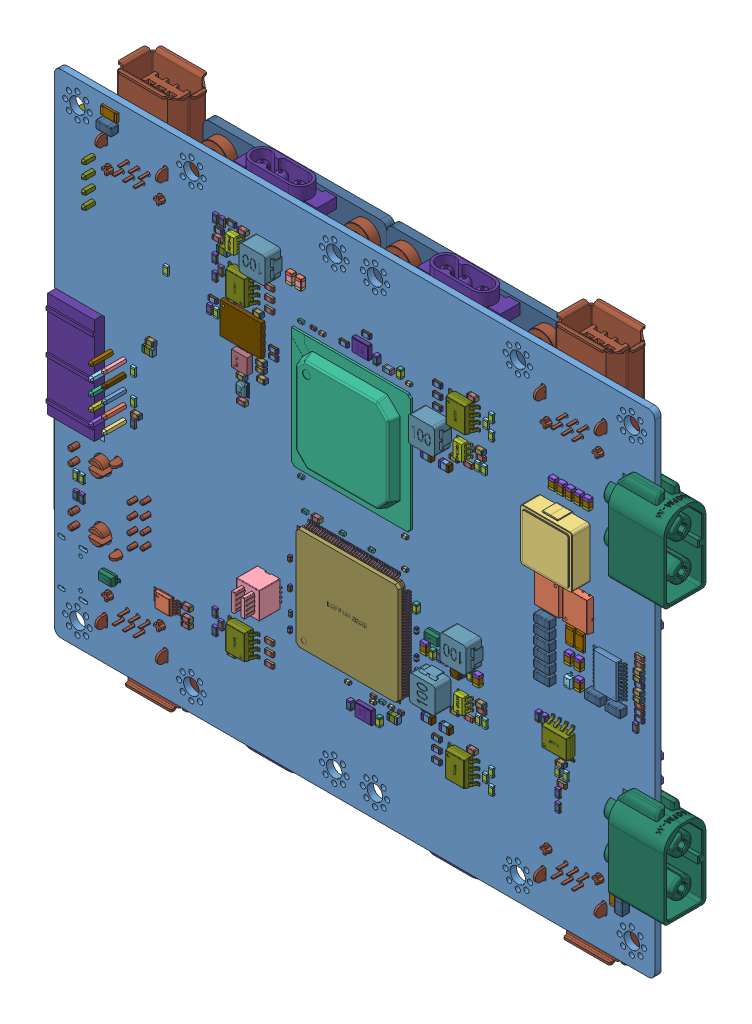
SolidWorks assembly Mother  Board, configuration 默认. Lengths in mm. (continued)
Components (placement in the parent): (continued)
- Mother  Board.step-1: Mother  Board.step [默认] at origin size (122.6 102.08 21) (continued)
  - C26.step-1: C26.step [默认] at origin size (1.6 0.8 0.8) (continued)
    - 5993854224.step-1: 5993854224.step [默认] at (32.3851 81.5341 0) x (1 0 0) z (0 0 1) size (1.6 0.8 0.8) (continued)
      - Terminal-17.step-1: Terminal-17.step [默认] at (-0.8 -0.4 0) size (1.6 0.8 0.8)
        - Open_CASCADE_STEP_translator_6.8_47.1.1-60.step-1: Open_CASCADE_STEP_translator_6.8_47.1.1-60.step [默认] at origin size (0.3 0.8 0.8)
        - Open_CASCADE_STEP_translator_6.8_47.1.2-61.step-1: Open_CASCADE_STEP_translator_6.8_47.1.2-61.step [默认] at origin size (0.3 0.8 0.8)
      - Mid_Body-8.step-1: Mid_Body-8.step [默认] at (-0.8 -0.4 0) size (1 0.8 0.8)
        - Open_CASCADE_STEP_translator_6.8_47.2.1-62.step-1: Open_CASCADE_STEP_translator_6.8_47.2.1-62.step [默认] at origin size (1 0.8 0.8)
  - C25.step-1: C25.step [默认] at origin size (2.01 1.25 0.94)
    - 5993850544.step-1: 5993850544.step [默认] at (28.7019 76.5809 0) x (-1 0 0) z (0 0 1) size (2.01 1.25 0.94)
      - Fillet1-63.step-1: Fillet1-63.step [默认] at origin size (0.5 1.25 0.94)
      - Fillet2-64.step-1: Fillet2-64.step [默认] at origin size (0.5 1.25 0.94)
      - body2-65.step-1: body2-65.step [默认] at origin size (1.01 1.22 0.92)
  - C24.step-1: C24.step [默认] at origin size (1.6 0.8 0.8)
    - 5993853264.step-1: 5993853264.step [默认] at (73.4059 21.8439 0) x (-1 0 0) z (0 0 1) size (1.6 0.8 0.8)
      - Terminal-6.step-1: Terminal-6.step [默认] at (-0.8 -0.4 0) size (1.6 0.8 0.8)
        - Open_CASCADE_STEP_translator_6.8_47.1.1-10.step-1: Open_CASCADE_STEP_translator_6.8_47.1.1-10.step [默认] at origin size (0.3 0.8 0.8)
        - Open_CASCADE_STEP_translator_6.8_47.1.2-11.step-1: Open_CASCADE_STEP_translator_6.8_47.1.2-11.step [默认] at origin size (0.3 0.8 0.8)
      - Mid_Body-5.step-1: Mid_Body-5.step [默认] at (-0.8 -0.4 0) size (1 0.8 0.8)
        - Open_CASCADE_STEP_translator_6.8_47.2.1-12.step-1: Open_CASCADE_STEP_translator_6.8_47.2.1-12.step [默认] at origin size (1 0.8 0.8)
  - C23.step-1: C23.step [默认] at origin size (2.01 1.25 0.94)
    - 5993850784.step-1: 5993850784.step [默认] at (71.6281 18.1611 0) x (1 0 0) z (0 0 1) size (2.01 1.25 0.94)
      - Fillet1.step-1: Fillet1.step [默认] at origin size (0.5 1.25 0.94)
      - Fillet2.step-1: Fillet2.step [默认] at origin size (0.5 1.25 0.94)
      - body2.step-1: body2.step [默认] at origin size (1.01 1.22 0.92)
  - C21.step-1: C21.step [默认] at origin size (2.01 1.25 0.94)
    - 5993850784.step-1: 5993850784.step [默认] at (68.0721 63.6271 0) x (1 0 0) z (0 0 1) size (2.01 1.25 0.94)
      - Fillet1.step-1: Fillet1.step [默认] at origin size (0.5 1.25 0.94)
      - Fillet2.step-1: Fillet2.step [默认] at origin size (0.5 1.25 0.94)
      - body2.step-1: body2.step [默认] at origin size (1.01 1.22 0.92)
  - C19.step-1: C19.step [默认] at origin size (1.25 2.01 0.94)
    - 5993850384.step-1: 5993850384.step [默认] at (43.4341 78.4859 0) x (0 -1 0) z (0 0 1) size (2.01 1.25 0.94)
      - Fillet1-51.step-1: Fillet1-51.step [默认] at origin size (0.5 1.25 0.94)
      - Fillet2-52.step-1: Fillet2-52.step [默认] at origin size (0.5 1.25 0.94)
      - body2-53.step-1: body2-53.step [默认] at origin size (1.01 1.22 0.92)
  - C17.step-1: C17.step [默认] at origin size (2.01 1.25 0.94)
    - 5993850784.step-1: 5993850784.step [默认] at (68.1991 18.1611 0) x (1 0 0) z (0 0 1) size (2.01 1.25 0.94)
      - Fillet1.step-1: Fillet1.step [默认] at origin size (0.5 1.25 0.94)
      - Fillet2.step-1: Fillet2.step [默认] at origin size (0.5 1.25 0.94)
      - body2.step-1: body2.step [默认] at origin size (1.01 1.22 0.92)
  - C16.step-1: C16.step [默认] at origin size (1.6 0.8 0.8)
    - 5993853264.step-1: 5993853264.step [默认] at (78.1049 67.6909 0) x (-1 0 0) z (0 0 1) size (1.6 0.8 0.8)
      - Terminal-6.step-1: Terminal-6.step [默认] at (-0.8 -0.4 0) size (1.6 0.8 0.8)
        - Open_CASCADE_STEP_translator_6.8_47.1.1-10.step-1: Open_CASCADE_STEP_translator_6.8_47.1.1-10.step [默认] at origin size (0.3 0.8 0.8)
        - Open_CASCADE_STEP_translator_6.8_47.1.2-11.step-1: Open_CASCADE_STEP_translator_6.8_47.1.2-11.step [默认] at origin size (0.3 0.8 0.8)
      - Mid_Body-5.step-1: Mid_Body-5.step [默认] at (-0.8 -0.4 0) size (1 0.8 0.8)
        - Open_CASCADE_STEP_translator_6.8_47.2.1-12.step-1: Open_CASCADE_STEP_translator_6.8_47.2.1-12.step [默认] at origin size (1 0.8 0.8)
  - C15.step-1: C15.step [默认] at origin size (1.6 0.8 0.8)
    - 5993854224.step-1: 5993854224.step [默认] at (27.5591 77.9781 0) x (1 0 0) z (0 0 1) size (1.6 0.8 0.8)
      - Terminal-17.step-1: Terminal-17.step [默认] at (-0.8 -0.4 0) size (1.6 0.8 0.8)
        - Open_CASCADE_STEP_translator_6.8_47.1.1-60.step-1: Open_CASCADE_STEP_translator_6.8_47.1.1-60.step [默认] at origin size (0.3 0.8 0.8)
        - Open_CASCADE_STEP_translator_6.8_47.1.2-61.step-1: Open_CASCADE_STEP_translator_6.8_47.1.2-61.step [默认] at origin size (0.3 0.8 0.8)
      - Mid_Body-8.step-1: Mid_Body-8.step [默认] at (-0.8 -0.4 0) size (1 0.8 0.8)
        - Open_CASCADE_STEP_translator_6.8_47.2.1-62.step-1: Open_CASCADE_STEP_translator_6.8_47.2.1-62.step [默认] at origin size (1 0.8 0.8)
  - C14.step-1: C14.step [默认] at origin size (1.6 0.8 0.8)
    - 5993853264.step-1: 5993853264.step [默认] at (78.2319 25.3999 0) x (-1 0 0) z (0 0 1) size (1.6 0.8 0.8)
      - Terminal-6.step-1: Terminal-6.step [默认] at (-0.8 -0.4 0) size (1.6 0.8 0.8)
        - Open_CASCADE_STEP_translator_6.8_47.1.1-10.step-1: Open_CASCADE_STEP_translator_6.8_47.1.1-10.step [默认] at origin size (0.3 0.8 0.8)
        - Open_CASCADE_STEP_translator_6.8_47.1.2-11.step-1: Open_CASCADE_STEP_translator_6.8_47.1.2-11.step [默认] at origin size (0.3 0.8 0.8)
      - Mid_Body-5.step-1: Mid_Body-5.step [默认] at (-0.8 -0.4 0) size (1 0.8 0.8)
        - Open_CASCADE_STEP_translator_6.8_47.2.1-12.step-1: Open_CASCADE_STEP_translator_6.8_47.2.1-12.step [默认] at origin size (1 0.8 0.8)
  - X1.step-1: X1.step [默认] at origin size (3.2 2.5 0.8)
    - XTAL-3225.step-1: XTAL-3225.step [默认] at (23.9389 30.1217 -1.2164) x (0 -1 0) z (1 0 0) size (2.5 0.8 3.2)
  - U12.step-1: U12.step [默认] at origin size (5.03 3.01 1.05)
    - User_Library-MSOP-10-1.step-1: User_Library-MSOP-10-1.step [默认] at (17.3989 12.0603 0) x (0 -1 0) z (-1 0 0) size (3.01 1.05 5.03)
  - U11.step-1: U11.step [默认] at origin size (4.02 4.02 1.08)
    - User_Library-QFN24_4x4.step-1: User_Library-QFN24_4x4.step [默认] at (21.844 21.3359 -1.2164) x (0 -1 0) z (0 0 -1) size (4.02 4.02 1.08)
      - Imported.step-1: Imported.step [默认] at origin size (2.5 2.5 0.02)
      - Imported_2.step-1: Imported_2.step [默认] at origin size (0.42 0.25 0.1)
      - Imported_3.step-1: Imported_3.step [默认] at origin size (0.42 0.25 0.1)
      - Imported_4.step-1: Imported_4.step [默认] at origin size (0.42 0.25 0.1)
      - Imported_5.step-1: Imported_5.step [默认] at origin size (0.42 0.25 0.1)
      - Imported_6.step-1: Imported_6.step [默认] at origin size (0.42 0.25 0.1)
      - Imported_7.step-1: Imported_7.step [默认] at origin size (0.42 0.25 0.1)
      - Imported_8.step-1: Imported_8.step [默认] at origin size (0.42 0.25 0.1)
      - Imported_9.step-1: Imported_9.step [默认] at origin size (0.42 0.25 0.1)
      - Imported_10.step-1: Imported_10.step [默认] at origin size (0.42 0.25 0.1)
      - Imported_11.step-1: Imported_11.step [默认] at origin size (0.42 0.25 0.1)
      - Imported_12.step-1: Imported_12.step [默认] at origin size (0.42 0.25 0.1)
      - Imported_13.step-1: Imported_13.step [默认] at origin size (0.42 0.25 0.1)
      - Imported_14.step-1: Imported_14.step [默认] at origin size (0.25 0.42 0.1)
      - Imported_15.step-1: Imported_15.step [默认] at origin size (0.25 0.42 0.1)
      - Imported_16.step-1: Imported_16.step [默认] at origin size (0.25 0.42 0.1)
      - Imported_17.step-1: Imported_17.step [默认] at origin size (0.25 0.42 0.1)
      - Imported_18.step-1: Imported_18.step [默认] at origin size (0.25 0.42 0.1)
      - Imported_19.step-1: Imported_19.step [默认] at origin size (0.25 0.42 0.1)
      - Imported_20.step-1: Imported_20.step [默认] at origin size (0.25 0.42 0.1)
      - Imported_21.step-1: Imported_21.step [默认] at origin size (0.25 0.42 0.1)
      - Imported_22.step-1: Imported_22.step [默认] at origin size (0.25 0.42 0.1)
      - Imported_23.step-1: Imported_23.step [默认] at origin size (0.25 0.42 0.1)
      - Imported_24.step-1: Imported_24.step [默认] at origin size (0.25 0.42 0.1)
      - Imported_25.step-1: Imported_25.step [默认] at origin size (0.25 0.42 0.1)
      - Imported_26.step-1: Imported_26.step [默认] at origin size (4 4 0.08)
      - Imported_27.step-1: Imported_27.step [默认] at origin size (3.85 3.85 0.9)
      - Imported_28.step-1: Imported_28.step [默认] at origin size (0.48 0.46 1.02)
  - U9.step-1: U9.step [默认] at origin size (3.02 3.02 1.05)
    - User_Library-MPU9250.step-1: User_Library-MPU9250.step [默认] at (32.2581 59.8168 0.03) x (0 -1 0) z (-1 0 0) size (3.02 1.05 3.02)
  - U8.step-1: U8.step [默认] at origin size (2 2.5 1)
    - User_Library-BST-BMP280.step-1: User_Library-BST-BMP280.step [默认] at (32.2581 55.1181 0) x (0 1 0) z (1 0 0) size (2.5 1 2)
  - U7.step-1: U7.step [默认] at origin size (5 6.01 1.9)
    - SOP8.step-1: SOP8.step [默认] at (93.809 27.432 0) x (0 1 0) z (0 0 1) size (6.01 5 1.9)
      - LOGO_-69.step-1: LOGO_-69.step [默认] at (0.0116 0 0.095) x (0 -1 0) z (0 0 -1) size (1.5 1.73 0.01)
      - SOP8-70.step-1: SOP8-70.step [默认] at origin size (6.01 5 1.9)
  - U6.step-1: U6.step [默认] at origin size (2.8 2.9 1.1)
    - User_Library-SOT23-5.step-1: User_Library-SOT23-5.step [默认] at (74.6706 27.9029 -0.15) x (0 1 0) z (1 0 0) size (2.9 1.1 2.8)
      - User_Library-SOT23-5_SOT23-5_Connector_Default.step-1: User_Library-SOT23-5_SOT23-5_Connector_Default.step [默认] at (0.2717 0.137 -1.6839) x (0 0 -1) z (1 0 0) size (0.6 0.85 0.43)
      - User_Library-SOT23-5_SOT23-5_Connector_Default.step-2: User_Library-SOT23-5_SOT23-5_Connector_Default.step [默认] at (2.1716 0.137 -1.6839) x (0 0 -1) z (1 0 0) size (0.6 0.85 0.43)
      - User_Library-SOT23-5_SOT23-5_Connector_Default.step-3: User_Library-SOT23-5_SOT23-5_Connector_Default.step [默认] at (2.597 0.137 -0.0849) x (0 0 1) z (-1 0 0) size (0.6 0.85 0.43)
      - User_Library-SOT23-5_SOT23-5_Connector_Default.step-4: User_Library-SOT23-5_SOT23-5_Connector_Default.step [默认] at (0.6971 0.137 -0.0849) x (0 0 1) z (-1 0 0) size (0.6 0.85 0.43)
      - User_Library-SOT23-5_SOT23-5_Connector_Default.step-5: User_Library-SOT23-5_SOT23-5_Connector_Default.step [默认] at (1.2216 0.137 -1.6839) x (0 0 -1) z (1 0 0) size (0.6 0.85 0.43)
      - User_Library-SOT23-5_SOT23-5_Body_Default.step-1: User_Library-SOT23-5_SOT23-5_Body_Default.step [默认] at (-0.0154 0.137 -0.0849) size (2.9 1.1 1.6)
  - U2.step-1: U2.step [默认] at origin size (6.4 6.62 1.1)
    - 5993850064.step-1: 5993850064.step [默认] at (102.87 42.799 0) x (-1 0 0) z (0 0 1) size (6.4 6.62 1.1)
  - U1_D4.step-1: U1_D4.step [默认] at origin size (6.01 5 1.9)
    - SOP8.step-1: SOP8.step [默认] at (74.803 72.644 0) x (1 0 0) z (0 0 1) size (6.01 5 1.9)
      - LOGO_-69.step-1: LOGO_-69.step [默认] at (0.0116 0 0.095) x (0 -1 0) z (0 0 -1) size (1.5 1.73 0.01)
      - SOP8-70.step-1: SOP8-70.step [默认] at origin size (6.01 5 1.9)
  - U1_D3.step-1: U1_D3.step [默认] at origin size (6.01 5 1.9)
    - SOP8.step-1: SOP8.step [默认] at (32.258 72.6439 0) x (-1 0 0) z (0 0 1) size (6.01 5 1.9)
      - LOGO_-69.step-1: LOGO_-69.step [默认] at (0.0116 0 0.095) x (0 -1 0) z (0 0 -1) size (1.5 1.73 0.01)
      - SOP8-70.step-1: SOP8-70.step [默认] at origin size (6.01 5 1.9)
  - U1_D2.step-1: U1_D2.step [默认] at origin size (6.01 5 1.9)
    - SOP8.step-1: SOP8.step [默认] at (74.6761 13.462 0) x (1 0 0) z (0 0 1) size (6.01 5 1.9)
      - LOGO_-69.step-1: LOGO_-69.step [默认] at (0.0116 0 0.095) x (0 -1 0) z (0 0 -1) size (1.5 1.73 0.01)
      - SOP8-70.step-1: SOP8-70.step [默认] at origin size (6.01 5 1.9)
  - U1_D1.step-1: U1_D1.step [默认] at origin size (6.01 5 1.9)
    - SOP8.step-1: SOP8.step [默认] at (32.258 13.462 0) x (-1 0 0) z (0 0 1) size (6.01 5 1.9)
      - LOGO_-69.step-1: LOGO_-69.step [默认] at (0.0116 0 0.095) x (0 -1 0) z (0 0 -1) size (1.5 1.73 0.01)
      - SOP8-70.step-1: SOP8-70.step [默认] at origin size (6.01 5 1.9)
  - RS2.step-1: RS2.step [默认] at origin size (1.55 3.1 0.47)
    - User_Library-R1206.step-1: User_Library-R1206.step [默认] at (95.3701 45.3909 0) x (0 1 0) z (0 0 1) size (3.1 1.55 0.47)
  - RS1.step-1: RS1.step [默认] at origin size (1.55 3.1 0.47)
    - User_Library-R1206.step-1: User_Library-R1206.step [默认] at (97.2751 45.3909 0) x (0 1 0) z (0 0 1) size (3.1 1.55 0.47)
  - R44.step-1: R44.step [默认] at origin size (0.8 1.6 0.45)
    - 5993842864.step-1: 5993842864.step [默认] at (19.5578 25.5315 -1.2164) x (0 -1 0) z (0 0 -1) size (1.6 0.8 0.45)
      - Terminal-12.step-1: Terminal-12.step [默认] at (-0.8 -0.4 0) size (0.3 0.8 0.45)
        - Open_CASCADE_STEP_translator_6.8_21.2.1-28.step-1: Open_CASCADE_STEP_translator_6.8_21.2.1-28.step [默认] at origin size (0.3 0.8 0.45)
      - Terminal-12.step-2: Terminal-12.step [默认] at (0.8 0.4 0) x (-1 0 0) z (0 0 1) size (0.3 0.8 0.45)
        - Open_CASCADE_STEP_translator_6.8_21.2.1-28.step-1: Open_CASCADE_STEP_translator_6.8_21.2.1-28.step [默认] at origin size (0.3 0.8 0.45)
      - Mid_Body-29.step-1: Mid_Body-29.step [默认] at (-0.8 -0.4 0) size (1.51 0.8 0.36)
      - Mark-30.step-1: Mark-30.step [默认] at (-0.5 -0.4 0.405) size (1 0.8 0.05)
  - R43.step-1: R43.step [默认] at origin size (1.6 0.8 0.45)
    - 5993853584.step-1: 5993853584.step [默认] at (23.7491 17.9069 -1.2164) x (1 0 0) z (0 0 -1) size (1.6 0.8 0.45)
      - Terminal-1.step-1: Terminal-1.step [默认] at (-0.8 -0.4 0) size (0.3 0.8 0.45)
        - Open_CASCADE_STEP_translator_6.8_21.2.1.step-1: Open_CASCADE_STEP_translator_6.8_21.2.1.step [默认] at origin size (0.3 0.8 0.45)
      - Terminal-1.step-2: Terminal-1.step [默认] at (0.8 0.4 0) x (-1 0 0) z (0 0 1) size (0.3 0.8 0.45)
        - Open_CASCADE_STEP_translator_6.8_21.2.1.step-1: Open_CASCADE_STEP_translator_6.8_21.2.1.step [默认] at origin size (0.3 0.8 0.45)
      - Mid_Body-0.step-1: Mid_Body-0.step [默认] at (-0.8 -0.4 0) size (1.51 0.8 0.36)
      - Mark.step-1: Mark.step [默认] at (-0.5 -0.4 0.405) size (1 0.8 0.05)
  - R42.step-1: R42.step [默认] at origin size (1.6 0.8 0.45)
    - 5993842944.step-1: 5993842944.step [默认] at (26.0349 19.9391 -1.2164) x (-1 0 0) z (0 0 -1) size (1.6 0.8 0.45)
      - Terminal-14.step-1: Terminal-14.step [默认] at (-0.8 -0.4 0) size (0.3 0.8 0.45)
        - Open_CASCADE_STEP_translator_6.8_21.2.1-34.step-1: Open_CASCADE_STEP_translator_6.8_21.2.1-34.step [默认] at origin size (0.3 0.8 0.45)
      - Terminal-14.step-2: Terminal-14.step [默认] at (0.8 0.4 0) x (-1 0 0) z (0 0 1) size (0.3 0.8 0.45)
        - Open_CASCADE_STEP_translator_6.8_21.2.1-34.step-1: Open_CASCADE_STEP_translator_6.8_21.2.1-34.step [默认] at origin size (0.3 0.8 0.45)
      - Mid_Body-35.step-1: Mid_Body-35.step [默认] at (-0.8 -0.4 0) size (1.51 0.8 0.36)
      - Mark-36.step-1: Mark-36.step [默认] at (-0.5 -0.4 0.405) size (1 0.8 0.05)
  - R41.step-1: R41.step [默认] at origin size (1.6 0.8 0.45)
    - 5993842944.step-1: 5993842944.step [默认] at (22.4788 26.4207 -1.2164) x (-1 0 0) z (0 0 -1) size (1.6 0.8 0.45)
      - Terminal-14.step-1: Terminal-14.step [默认] at (-0.8 -0.4 0) size (0.3 0.8 0.45)
        - Open_CASCADE_STEP_translator_6.8_21.2.1-34.step-1: Open_CASCADE_STEP_translator_6.8_21.2.1-34.step [默认] at origin size (0.3 0.8 0.45)
      - Terminal-14.step-2: Terminal-14.step [默认] at (0.8 0.4 0) x (-1 0 0) z (0 0 1) size (0.3 0.8 0.45)
        - Open_CASCADE_STEP_translator_6.8_21.2.1-34.step-1: Open_CASCADE_STEP_translator_6.8_21.2.1-34.step [默认] at origin size (0.3 0.8 0.45)
      - Mid_Body-35.step-1: Mid_Body-35.step [默认] at (-0.8 -0.4 0) size (1.51 0.8 0.36)
      - Mark-36.step-1: Mark-36.step [默认] at (-0.5 -0.4 0.405) size (1 0.8 0.05)
  - R40.step-1: R40.step [默认] at origin size (0.8 1.6 0.45)
    - 5993842864.step-1: 5993842864.step [默认] at (1.1429 24.5111 0) x (0 1 0) z (0 0 1) size (1.6 0.8 0.45)
      - Terminal-12.step-1: Terminal-12.step [默认] at (-0.8 -0.4 0) size (0.3 0.8 0.45)
        - Open_CASCADE_STEP_translator_6.8_21.2.1-28.step-1: Open_CASCADE_STEP_translator_6.8_21.2.1-28.step [默认] at origin size (0.3 0.8 0.45)
      - Terminal-12.step-2: Terminal-12.step [默认] at (0.8 0.4 0) x (-1 0 0) z (0 0 1) size (0.3 0.8 0.45)
        - Open_CASCADE_STEP_translator_6.8_21.2.1-28.step-1: Open_CASCADE_STEP_translator_6.8_21.2.1-28.step [默认] at origin size (0.3 0.8 0.45)
      - Mid_Body-29.step-1: Mid_Body-29.step [默认] at (-0.8 -0.4 0) size (1.51 0.8 0.36)
      - Mark-30.step-1: Mark-30.step [默认] at (-0.5 -0.4 0.405) size (1 0.8 0.05)
  - R39.step-1: R39.step [默认] at origin size (0.8 1.6 0.45)
    - 5993842864.step-1: 5993842864.step [默认] at (-0.0001 24.5111 0) x (0 1 0) z (0 0 1) size (1.6 0.8 0.45)
      - Terminal-12.step-1: Terminal-12.step [默认] at (-0.8 -0.4 0) size (0.3 0.8 0.45)
        - Open_CASCADE_STEP_translator_6.8_21.2.1-28.step-1: Open_CASCADE_STEP_translator_6.8_21.2.1-28.step [默认] at origin size (0.3 0.8 0.45)
      - Terminal-12.step-2: Terminal-12.step [默认] at (0.8 0.4 0) x (-1 0 0) z (0 0 1) size (0.3 0.8 0.45)
        - Open_CASCADE_STEP_translator_6.8_21.2.1-28.step-1: Open_CASCADE_STEP_translator_6.8_21.2.1-28.step [默认] at origin size (0.3 0.8 0.45)
      - Mid_Body-29.step-1: Mid_Body-29.step [默认] at (-0.8 -0.4 0) size (1.51 0.8 0.36)
      - Mark-30.step-1: Mark-30.step [默认] at (-0.5 -0.4 0.405) size (1 0.8 0.05)
  - R38.step-1: R38.step [默认] at origin size (0.8 1.6 0.45)
    - 5993842864.step-1: 5993842864.step [默认] at (16.5098 23.1186 -1.2164) x (0 -1 0) z (0 0 -1) size (1.6 0.8 0.45)
      - Terminal-12.step-1: Terminal-12.step [默认] at (-0.8 -0.4 0) size (0.3 0.8 0.45)
        - Open_CASCADE_STEP_translator_6.8_21.2.1-28.step-1: Open_CASCADE_STEP_translator_6.8_21.2.1-28.step [默认] at origin size (0.3 0.8 0.45)
      - Terminal-12.step-2: Terminal-12.step [默认] at (0.8 0.4 0) x (-1 0 0) z (0 0 1) size (0.3 0.8 0.45)
        - Open_CASCADE_STEP_translator_6.8_21.2.1-28.step-1: Open_CASCADE_STEP_translator_6.8_21.2.1-28.step [默认] at origin size (0.3 0.8 0.45)
      - Mid_Body-29.step-1: Mid_Body-29.step [默认] at (-0.8 -0.4 0) size (1.51 0.8 0.36)
      - Mark-30.step-1: Mark-30.step [默认] at (-0.5 -0.4 0.405) size (1 0.8 0.05)
  - R37.step-1: R37.step [默认] at origin size (0.8 1.6 0.45)
    - 5993843024.step-1: 5993843024.step [默认] at (16.5099 25.5317 -1.2164) x (0 1 0) z (0 0 -1) size (1.6 0.8 0.45)
      - Terminal-13.step-1: Terminal-13.step [默认] at (-0.8 -0.4 0) size (0.3 0.8 0.45)
        - Open_CASCADE_STEP_translator_6.8_21.2.1-31.step-1: Open_CASCADE_STEP_translator_6.8_21.2.1-31.step [默认] at origin size (0.3 0.8 0.45)
      - Terminal-13.step-2: Terminal-13.step [默认] at (0.8 0.4 0) x (-1 0 0) z (0 0 1) size (0.3 0.8 0.45)
        - Open_CASCADE_STEP_translator_6.8_21.2.1-31.step-1: Open_CASCADE_STEP_translator_6.8_21.2.1-31.step [默认] at origin size (0.3 0.8 0.45)
      - Mid_Body-32.step-1: Mid_Body-32.step [默认] at (-0.8 -0.4 0) size (1.51 0.8 0.36)
      - Mark-33.step-1: Mark-33.step [默认] at (-0.5 -0.4 0.405) size (1 0.8 0.05)
  - R36.step-1: R36.step [默认] at origin size (0.8 1.6 0.45)
    - 5993842864.step-1: 5993842864.step [默认] at (16.5098 17.1496 -1.2164) x (0 -1 0) z (0 0 -1) size (1.6 0.8 0.45)
      - Terminal-12.step-1: Terminal-12.step [默认] at (-0.8 -0.4 0) size (0.3 0.8 0.45)
        - Open_CASCADE_STEP_translator_6.8_21.2.1-28.step-1: Open_CASCADE_STEP_translator_6.8_21.2.1-28.step [默认] at origin size (0.3 0.8 0.45)
      - Terminal-12.step-2: Terminal-12.step [默认] at (0.8 0.4 0) x (-1 0 0) z (0 0 1) size (0.3 0.8 0.45)
        - Open_CASCADE_STEP_translator_6.8_21.2.1-28.step-1: Open_CASCADE_STEP_translator_6.8_21.2.1-28.step [默认] at origin size (0.3 0.8 0.45)
      - Mid_Body-29.step-1: Mid_Body-29.step [默认] at (-0.8 -0.4 0) size (1.51 0.8 0.36)
      - Mark-30.step-1: Mark-30.step [默认] at (-0.5 -0.4 0.405) size (1 0.8 0.05)
  - R35.step-1: R35.step [默认] at origin size (0.8 1.6 0.45)
    - 5993843024.step-1: 5993843024.step [默认] at (16.5099 19.5627 -1.2164) x (0 1 0) z (0 0 -1) size (1.6 0.8 0.45)
      - Terminal-13.step-1: Terminal-13.step [默认] at (-0.8 -0.4 0) size (0.3 0.8 0.45)
        - Open_CASCADE_STEP_translator_6.8_21.2.1-31.step-1: Open_CASCADE_STEP_translator_6.8_21.2.1-31.step [默认] at origin size (0.3 0.8 0.45)
      - Terminal-13.step-2: Terminal-13.step [默认] at (0.8 0.4 0) x (-1 0 0) z (0 0 1) size (0.3 0.8 0.45)
        - Open_CASCADE_STEP_translator_6.8_21.2.1-31.step-1: Open_CASCADE_STEP_translator_6.8_21.2.1-31.step [默认] at origin size (0.3 0.8 0.45)
      - Mid_Body-32.step-1: Mid_Body-32.step [默认] at (-0.8 -0.4 0) size (1.51 0.8 0.36)
      - Mark-33.step-1: Mark-33.step [默认] at (-0.5 -0.4 0.405) size (1 0.8 0.05)
  - R34.step-1: R34.step [默认] at origin size (0.8 1.6 0.45)
    - 5993843024.step-1: 5993843024.step [默认] at (1.1431 21.2089 0) x (0 -1 0) z (0 0 1) size (1.6 0.8 0.45)
      - Terminal-13.step-1: Terminal-13.step [默认] at (-0.8 -0.4 0) size (0.3 0.8 0.45)
        - Open_CASCADE_STEP_translator_6.8_21.2.1-31.step-1: Open_CASCADE_STEP_translator_6.8_21.2.1-31.step [默认] at origin size (0.3 0.8 0.45)
      - Terminal-13.step-2: Terminal-13.step [默认] at (0.8 0.4 0) x (-1 0 0) z (0 0 1) size (0.3 0.8 0.45)
        - Open_CASCADE_STEP_translator_6.8_21.2.1-31.step-1: Open_CASCADE_STEP_translator_6.8_21.2.1-31.step [默认] at origin size (0.3 0.8 0.45)
      - Mid_Body-32.step-1: Mid_Body-32.step [默认] at (-0.8 -0.4 0) size (1.51 0.8 0.36)
      - Mark-33.step-1: Mark-33.step [默认] at (-0.5 -0.4 0.405) size (1 0.8 0.05)
  - R33.step-1: R33.step [默认] at origin size (0.8 1.6 0.45)
    - 5993843024.step-1: 5993843024.step [默认] at (0.0001 21.2089 0) x (0 -1 0) z (0 0 1) size (1.6 0.8 0.45)
      - Terminal-13.step-1: Terminal-13.step [默认] at (-0.8 -0.4 0) size (0.3 0.8 0.45)
        - Open_CASCADE_STEP_translator_6.8_21.2.1-31.step-1: Open_CASCADE_STEP_translator_6.8_21.2.1-31.step [默认] at origin size (0.3 0.8 0.45)
      - Terminal-13.step-2: Terminal-13.step [默认] at (0.8 0.4 0) x (-1 0 0) z (0 0 1) size (0.3 0.8 0.45)
        - Open_CASCADE_STEP_translator_6.8_21.2.1-31.step-1: Open_CASCADE_STEP_translator_6.8_21.2.1-31.step [默认] at origin size (0.3 0.8 0.45)
      - Mid_Body-32.step-1: Mid_Body-32.step [默认] at (-0.8 -0.4 0) size (1.51 0.8 0.36)
      - Mark-33.step-1: Mark-33.step [默认] at (-0.5 -0.4 0.405) size (1 0.8 0.05)
  - R32.step-1: R32.step [默认] at origin size (0.8 1.6 0.45)
    - 5993842864.step-1: 5993842864.step [默认] at (94.4879 21.4631 0) x (0 1 0) z (0 0 1) size (1.6 0.8 0.45)
      - Terminal-12.step-1: Terminal-12.step [默认] at (-0.8 -0.4 0) size (0.3 0.8 0.45)
        - Open_CASCADE_STEP_translator_6.8_21.2.1-28.step-1: Open_CASCADE_STEP_translator_6.8_21.2.1-28.step [默认] at origin size (0.3 0.8 0.45)
      - Terminal-12.step-2: Terminal-12.step [默认] at (0.8 0.4 0) x (-1 0 0) z (0 0 1) size (0.3 0.8 0.45)
        - Open_CASCADE_STEP_translator_6.8_21.2.1-28.step-1: Open_CASCADE_STEP_translator_6.8_21.2.1-28.step [默认] at origin size (0.3 0.8 0.45)
      - Mid_Body-29.step-1: Mid_Body-29.step [默认] at (-0.8 -0.4 0) size (1.51 0.8 0.36)
      - Mark-30.step-1: Mark-30.step [默认] at (-0.5 -0.4 0.405) size (1 0.8 0.05)
  - R31.step-1: R31.step [默认] at origin size (1.6 0.8 0.45)
    - 5993842944.step-1: 5993842944.step [默认] at (93.7259 19.6849 0) x (-1 0 0) z (0 0 1) size (1.6 0.8 0.45)
      - Terminal-14.step-1: Terminal-14.step [默认] at (-0.8 -0.4 0) size (0.3 0.8 0.45)
        - Open_CASCADE_STEP_translator_6.8_21.2.1-34.step-1: Open_CASCADE_STEP_translator_6.8_21.2.1-34.step [默认] at origin size (0.3 0.8 0.45)
      - Terminal-14.step-2: Terminal-14.step [默认] at (0.8 0.4 0) x (-1 0 0) z (0 0 1) size (0.3 0.8 0.45)
        - Open_CASCADE_STEP_translator_6.8_21.2.1-34.step-1: Open_CASCADE_STEP_translator_6.8_21.2.1-34.step [默认] at origin size (0.3 0.8 0.45)
      - Mid_Body-35.step-1: Mid_Body-35.step [默认] at (-0.8 -0.4 0) size (1.51 0.8 0.36)
      - Mark-36.step-1: Mark-36.step [默认] at (-0.5 -0.4 0.405) size (1 0.8 0.05)
  - R28.step-1: R28.step [默认] at origin size (0.8 1.6 0.45)
    - 5993842864.step-1: 5993842864.step [默认] at (92.9639 21.4631 0) x (0 1 0) z (0 0 1) size (1.6 0.8 0.45)
      - Terminal-12.step-1: Terminal-12.step [默认] at (-0.8 -0.4 0) size (0.3 0.8 0.45)
        - Open_CASCADE_STEP_translator_6.8_21.2.1-28.step-1: Open_CASCADE_STEP_translator_6.8_21.2.1-28.step [默认] at origin size (0.3 0.8 0.45)
      - Terminal-12.step-2: Terminal-12.step [默认] at (0.8 0.4 0) x (-1 0 0) z (0 0 1) size (0.3 0.8 0.45)
        - Open_CASCADE_STEP_translator_6.8_21.2.1-28.step-1: Open_CASCADE_STEP_translator_6.8_21.2.1-28.step [默认] at origin size (0.3 0.8 0.45)
      - Mid_Body-29.step-1: Mid_Body-29.step [默认] at (-0.8 -0.4 0) size (1.51 0.8 0.36)
      - Mark-30.step-1: Mark-30.step [默认] at (-0.5 -0.4 0.405) size (1 0.8 0.05)
  - R30.step-1: R30.step [默认] at origin size (0.8 1.6 0.45)
    - 5993843024.step-1: 5993843024.step [默认] at (92.9641 17.9069 0) x (0 -1 0) z (0 0 1) size (1.6 0.8 0.45)
      - Terminal-13.step-1: Terminal-13.step [默认] at (-0.8 -0.4 0) size (0.3 0.8 0.45)
        - Open_CASCADE_STEP_translator_6.8_21.2.1-31.step-1: Open_CASCADE_STEP_translator_6.8_21.2.1-31.step [默认] at origin size (0.3 0.8 0.45)
      - Terminal-13.step-2: Terminal-13.step [默认] at (0.8 0.4 0) x (-1 0 0) z (0 0 1) size (0.3 0.8 0.45)
        - Open_CASCADE_STEP_translator_6.8_21.2.1-31.step-1: Open_CASCADE_STEP_translator_6.8_21.2.1-31.step [默认] at origin size (0.3 0.8 0.45)
      - Mid_Body-32.step-1: Mid_Body-32.step [默认] at (-0.8 -0.4 0) size (1.51 0.8 0.36)
      - Mark-33.step-1: Mark-33.step [默认] at (-0.5 -0.4 0.405) size (1 0.8 0.05)
  - R27.step-1: R27.step [默认] at origin size (0.8 1.6 0.45)
    - 5993842864.step-1: 5993842864.step [默认] at (71.2469 29.2101 0) x (0 1 0) z (0 0 1) size (1.6 0.8 0.45)
      - Terminal-12.step-1: Terminal-12.step [默认] at (-0.8 -0.4 0) size (0.3 0.8 0.45)
        - Open_CASCADE_STEP_translator_6.8_21.2.1-28.step-1: Open_CASCADE_STEP_translator_6.8_21.2.1-28.step [默认] at origin size (0.3 0.8 0.45)
      - Terminal-12.step-2: Terminal-12.step [默认] at (0.8 0.4 0) x (-1 0 0) z (0 0 1) size (0.3 0.8 0.45)
        - Open_CASCADE_STEP_translator_6.8_21.2.1-28.step-1: Open_CASCADE_STEP_translator_6.8_21.2.1-28.step [默认] at origin size (0.3 0.8 0.45)
      - Mid_Body-29.step-1: Mid_Body-29.step [默认] at (-0.8 -0.4 0) size (1.51 0.8 0.36)
      - Mark-30.step-1: Mark-30.step [默认] at (-0.5 -0.4 0.405) size (1 0.8 0.05)
  - R29.step-1: R29.step [默认] at origin size (0.8 1.6 0.45)
    - 5993843024.step-1: 5993843024.step [默认] at (92.9641 15.4939 0) x (0 -1 0) z (0 0 1) size (1.6 0.8 0.45)
      - Terminal-13.step-1: Terminal-13.step [默认] at (-0.8 -0.4 0) size (0.3 0.8 0.45)
        - Open_CASCADE_STEP_translator_6.8_21.2.1-31.step-1: Open_CASCADE_STEP_translator_6.8_21.2.1-31.step [默认] at origin size (0.3 0.8 0.45)
      - Terminal-13.step-2: Terminal-13.step [默认] at (0.8 0.4 0) x (-1 0 0) z (0 0 1) size (0.3 0.8 0.45)
        - Open_CASCADE_STEP_translator_6.8_21.2.1-31.step-1: Open_CASCADE_STEP_translator_6.8_21.2.1-31.step [默认] at origin size (0.3 0.8 0.45)
      - Mid_Body-32.step-1: Mid_Body-32.step [默认] at (-0.8 -0.4 0) size (1.51 0.8 0.36)
      - Mark-33.step-1: Mark-33.step [默认] at (-0.5 -0.4 0.405) size (1 0.8 0.05)
  - R26.step-1: R26.step [默认] at origin size (0.8 1.6 0.45)
    - 5993843024.step-1: 5993843024.step [默认] at (70.1041 29.2099 0) x (0 -1 0) z (0 0 1) size (1.6 0.8 0.45)
      - Terminal-13.step-1: Terminal-13.step [默认] at (-0.8 -0.4 0) size (0.3 0.8 0.45)
        - Open_CASCADE_STEP_translator_6.8_21.2.1-31.step-1: Open_CASCADE_STEP_translator_6.8_21.2.1-31.step [默认] at origin size (0.3 0.8 0.45)
      - Terminal-13.step-2: Terminal-13.step [默认] at (0.8 0.4 0) x (-1 0 0) z (0 0 1) size (0.3 0.8 0.45)
        - Open_CASCADE_STEP_translator_6.8_21.2.1-31.step-1: Open_CASCADE_STEP_translator_6.8_21.2.1-31.step [默认] at origin size (0.3 0.8 0.45)
      - Mid_Body-32.step-1: Mid_Body-32.step [默认] at (-0.8 -0.4 0) size (1.51 0.8 0.36)
      - Mark-33.step-1: Mark-33.step [默认] at (-0.5 -0.4 0.405) size (1 0.8 0.05)
  - R13.step-1: R13.step [默认] at origin size (1.6 0.8 0.45)
    - 5993842144.step-1: 5993842144.step [默认] at (108.7121 39.2431 0) x (1 0 0) z (0 0 1) size (1.6 0.8 0.45)
      - Terminal-10.step-1: Terminal-10.step [默认] at (-0.8 -0.4 0) size (0.3 0.8 0.45)
        - Open_CASCADE_STEP_translator_6.8_21.2.1-22.step-1: Open_CASCADE_STEP_translator_6.8_21.2.1-22.step [默认] at origin size (0.3 0.8 0.45)
      - Terminal-10.step-2: Terminal-10.step [默认] at (0.8 0.4 0) x (-1 0 0) z (0 0 1) size (0.3 0.8 0.45)
        - Open_CASCADE_STEP_translator_6.8_21.2.1-22.step-1: Open_CASCADE_STEP_translator_6.8_21.2.1-22.step [默认] at origin size (0.3 0.8 0.45)
      - Mid_Body-23.step-1: Mid_Body-23.step [默认] at (-0.8 -0.4 0) size (1.51 0.8 0.36)
      - Mark-24.step-1: Mark-24.step [默认] at (-0.5 -0.4 0.405) size (1 0.8 0.05)
  - R12.step-1: R12.step [默认] at origin size (1.6 0.8 0.45)
    - 5993842144.step-1: 5993842144.step [默认] at (108.7121 38.1001 0) x (1 0 0) z (0 0 1) size (1.6 0.8 0.45)
      - Terminal-10.step-1: Terminal-10.step [默认] at (-0.8 -0.4 0) size (0.3 0.8 0.45)
        - Open_CASCADE_STEP_translator_6.8_21.2.1-22.step-1: Open_CASCADE_STEP_translator_6.8_21.2.1-22.step [默认] at origin size (0.3 0.8 0.45)
      - Terminal-10.step-2: Terminal-10.step [默认] at (0.8 0.4 0) x (-1 0 0) z (0 0 1) size (0.3 0.8 0.45)
        - Open_CASCADE_STEP_translator_6.8_21.2.1-22.step-1: Open_CASCADE_STEP_translator_6.8_21.2.1-22.step [默认] at origin size (0.3 0.8 0.45)
      - Mid_Body-23.step-1: Mid_Body-23.step [默认] at (-0.8 -0.4 0) size (1.51 0.8 0.36)
      - Mark-24.step-1: Mark-24.step [默认] at (-0.5 -0.4 0.405) size (1 0.8 0.05)
  - R11.step-1: R11.step [默认] at origin size (1.6 0.8 0.45)
    - 5993842144.step-1: 5993842144.step [默认] at (108.7121 43.8151 0) x (1 0 0) z (0 0 1) size (1.6 0.8 0.45)
      - Terminal-10.step-1: Terminal-10.step [默认] at (-0.8 -0.4 0) size (0.3 0.8 0.45)
        - Open_CASCADE_STEP_translator_6.8_21.2.1-22.step-1: Open_CASCADE_STEP_translator_6.8_21.2.1-22.step [默认] at origin size (0.3 0.8 0.45)
      - Terminal-10.step-2: Terminal-10.step [默认] at (0.8 0.4 0) x (-1 0 0) z (0 0 1) size (0.3 0.8 0.45)
        - Open_CASCADE_STEP_translator_6.8_21.2.1-22.step-1: Open_CASCADE_STEP_translator_6.8_21.2.1-22.step [默认] at origin size (0.3 0.8 0.45)
      - Mid_Body-23.step-1: Mid_Body-23.step [默认] at (-0.8 -0.4 0) size (1.51 0.8 0.36)
      - Mark-24.step-1: Mark-24.step [默认] at (-0.5 -0.4 0.405) size (1 0.8 0.05)
  - R10.step-1: R10.step [默认] at origin size (1.6 0.8 0.45)
    - 5993842944.step-1: 5993842944.step [默认] at (108.7119 47.2439 0) x (-1 0 0) z (0 0 1) size (1.6 0.8 0.45)
      - Terminal-14.step-1: Terminal-14.step [默认] at (-0.8 -0.4 0) size (0.3 0.8 0.45)
        - Open_CASCADE_STEP_translator_6.8_21.2.1-34.step-1: Open_CASCADE_STEP_translator_6.8_21.2.1-34.step [默认] at origin size (0.3 0.8 0.45)
      - Terminal-14.step-2: Terminal-14.step [默认] at (0.8 0.4 0) x (-1 0 0) z (0 0 1) size (0.3 0.8 0.45)
        - Open_CASCADE_STEP_translator_6.8_21.2.1-34.step-1: Open_CASCADE_STEP_translator_6.8_21.2.1-34.step [默认] at origin size (0.3 0.8 0.45)
      - Mid_Body-35.step-1: Mid_Body-35.step [默认] at (-0.8 -0.4 0) size (1.51 0.8 0.36)
      - Mark-36.step-1: Mark-36.step [默认] at (-0.5 -0.4 0.405) size (1 0.8 0.05)
  - R9.step-1: R9.step [默认] at origin size (1.6 0.8 0.45)
    - 5993842944.step-1: 5993842944.step [默认] at (108.7119 48.3869 0) x (-1 0 0) z (0 0 1) size (1.6 0.8 0.45)
      - Terminal-14.step-1: Terminal-14.step [默认] at (-0.8 -0.4 0) size (0.3 0.8 0.45)
        - Open_CASCADE_STEP_translator_6.8_21.2.1-34.step-1: Open_CASCADE_STEP_translator_6.8_21.2.1-34.step [默认] at origin size (0.3 0.8 0.45)
      - Terminal-14.step-2: Terminal-14.step [默认] at (0.8 0.4 0) x (-1 0 0) z (0 0 1) size (0.3 0.8 0.45)
        - Open_CASCADE_STEP_translator_6.8_21.2.1-34.step-1: Open_CASCADE_STEP_translator_6.8_21.2.1-34.step [默认] at origin size (0.3 0.8 0.45)
      - Mid_Body-35.step-1: Mid_Body-35.step [默认] at (-0.8 -0.4 0) size (1.51 0.8 0.36)
      - Mark-36.step-1: Mark-36.step [默认] at (-0.5 -0.4 0.405) size (1 0.8 0.05)
  - R8.step-1: R8.step [默认] at origin size (0.8 1.6 0.45)
    - 5993843024.step-1: 5993843024.step [默认] at (107.9501 36.3219 0) x (0 -1 0) z (0 0 1) size (1.6 0.8 0.45)
      - Terminal-13.step-1: Terminal-13.step [默认] at (-0.8 -0.4 0) size (0.3 0.8 0.45)
        - Open_CASCADE_STEP_translator_6.8_21.2.1-31.step-1: Open_CASCADE_STEP_translator_6.8_21.2.1-31.step [默认] at origin size (0.3 0.8 0.45)
      - Terminal-13.step-2: Terminal-13.step [默认] at (0.8 0.4 0) x (-1 0 0) z (0 0 1) size (0.3 0.8 0.45)
        - Open_CASCADE_STEP_translator_6.8_21.2.1-31.step-1: Open_CASCADE_STEP_translator_6.8_21.2.1-31.step [默认] at origin size (0.3 0.8 0.45)
      - Mid_Body-32.step-1: Mid_Body-32.step [默认] at (-0.8 -0.4 0) size (1.51 0.8 0.36)
      - Mark-33.step-1: Mark-33.step [默认] at (-0.5 -0.4 0.405) size (1 0.8 0.05)
  - R7.step-1: R7.step [默认] at origin size (1.6 0.8 0.45)
    - 5993842944.step-1: 5993842944.step [默认] at (108.7119 40.3859 0) x (-1 0 0) z (0 0 1) size (1.6 0.8 0.45)
      - Terminal-14.step-1: Terminal-14.step [默认] at (-0.8 -0.4 0) size (0.3 0.8 0.45)
        - Open_CASCADE_STEP_translator_6.8_21.2.1-34.step-1: Open_CASCADE_STEP_translator_6.8_21.2.1-34.step [默认] at origin size (0.3 0.8 0.45)
      - Terminal-14.step-2: Terminal-14.step [默认] at (0.8 0.4 0) x (-1 0 0) z (0 0 1) size (0.3 0.8 0.45)
        - Open_CASCADE_STEP_translator_6.8_21.2.1-34.step-1: Open_CASCADE_STEP_translator_6.8_21.2.1-34.step [默认] at origin size (0.3 0.8 0.45)
      - Mid_Body-35.step-1: Mid_Body-35.step [默认] at (-0.8 -0.4 0) size (1.51 0.8 0.36)
      - Mark-36.step-1: Mark-36.step [默认] at (-0.5 -0.4 0.405) size (1 0.8 0.05)
  - R63.step-1: R63.step [默认] at origin size (0.8 1.6 0.45)
    - 5993842864.step-1: 5993842864.step [默认] at (17.3989 67.4371 0) x (0 1 0) z (0 0 1) size (1.6 0.8 0.45)
      - Terminal-12.step-1: Terminal-12.step [默认] at (-0.8 -0.4 0) size (0.3 0.8 0.45)
        - Open_CASCADE_STEP_translator_6.8_21.2.1-28.step-1: Open_CASCADE_STEP_translator_6.8_21.2.1-28.step [默认] at origin size (0.3 0.8 0.45)
      - Terminal-12.step-2: Terminal-12.step [默认] at (0.8 0.4 0) x (-1 0 0) z (0 0 1) size (0.3 0.8 0.45)
        - Open_CASCADE_STEP_translator_6.8_21.2.1-28.step-1: Open_CASCADE_STEP_translator_6.8_21.2.1-28.step [默认] at origin size (0.3 0.8 0.45)
      - Mid_Body-29.step-1: Mid_Body-29.step [默认] at (-0.8 -0.4 0) size (1.51 0.8 0.36)
      - Mark-30.step-1: Mark-30.step [默认] at (-0.5 -0.4 0.405) size (1 0.8 0.05)
  - R6_D4.step-1: R6_D4.step [默认] at origin size (0.8 1.6 0.45)
    - 5993842864.step-1: 5993842864.step [默认] at (80.1369 71.1201 0) x (0 1 0) z (0 0 1) size (1.6 0.8 0.45)
      - Terminal-12.step-1: Terminal-12.step [默认] at (-0.8 -0.4 0) size (0.3 0.8 0.45)
        - Open_CASCADE_STEP_translator_6.8_21.2.1-28.step-1: Open_CASCADE_STEP_translator_6.8_21.2.1-28.step [默认] at origin size (0.3 0.8 0.45)
      - Terminal-12.step-2: Terminal-12.step [默认] at (0.8 0.4 0) x (-1 0 0) z (0 0 1) size (0.3 0.8 0.45)
        - Open_CASCADE_STEP_translator_6.8_21.2.1-28.step-1: Open_CASCADE_STEP_translator_6.8_21.2.1-28.step [默认] at origin size (0.3 0.8 0.45)
      - Mid_Body-29.step-1: Mid_Body-29.step [默认] at (-0.8 -0.4 0) size (1.51 0.8 0.36)
      - Mark-30.step-1: Mark-30.step [默认] at (-0.5 -0.4 0.405) size (1 0.8 0.05)
  - R6_D3.step-1: R6_D3.step [默认] at origin size (0.8 1.6 0.45)
    - 5993843024.step-1: 5993843024.step [默认] at (26.7971 74.1679 0) x (0 -1 0) z (0 0 1) size (1.6 0.8 0.45)
      - Terminal-13.step-1: Terminal-13.step [默认] at (-0.8 -0.4 0) size (0.3 0.8 0.45)
        - Open_CASCADE_STEP_translator_6.8_21.2.1-31.step-1: Open_CASCADE_STEP_translator_6.8_21.2.1-31.step [默认] at origin size (0.3 0.8 0.45)
      - Terminal-13.step-2: Terminal-13.step [默认] at (0.8 0.4 0) x (-1 0 0) z (0 0 1) size (0.3 0.8 0.45)
        - Open_CASCADE_STEP_translator_6.8_21.2.1-31.step-1: Open_CASCADE_STEP_translator_6.8_21.2.1-31.step [默认] at origin size (0.3 0.8 0.45)
      - Mid_Body-32.step-1: Mid_Body-32.step [默认] at (-0.8 -0.4 0) size (1.51 0.8 0.36)
      - Mark-33.step-1: Mark-33.step [默认] at (-0.5 -0.4 0.405) size (1 0.8 0.05)
  - R6_D2.step-1: R6_D2.step [默认] at origin size (0.8 1.6 0.45)
    - 5993842864.step-1: 5993842864.step [默认] at (80.1369 11.9381 0) x (0 1 0) z (0 0 1) size (1.6 0.8 0.45)
      - Terminal-12.step-1: Terminal-12.step [默认] at (-0.8 -0.4 0) size (0.3 0.8 0.45)
        - Open_CASCADE_STEP_translator_6.8_21.2.1-28.step-1: Open_CASCADE_STEP_translator_6.8_21.2.1-28.step [默认] at origin size (0.3 0.8 0.45)
      - Terminal-12.step-2: Terminal-12.step [默认] at (0.8 0.4 0) x (-1 0 0) z (0 0 1) size (0.3 0.8 0.45)
        - Open_CASCADE_STEP_translator_6.8_21.2.1-28.step-1: Open_CASCADE_STEP_translator_6.8_21.2.1-28.step [默认] at origin size (0.3 0.8 0.45)
      - Mid_Body-29.step-1: Mid_Body-29.step [默认] at (-0.8 -0.4 0) size (1.51 0.8 0.36)
      - Mark-30.step-1: Mark-30.step [默认] at (-0.5 -0.4 0.405) size (1 0.8 0.05)
  - R6_D1.step-1: R6_D1.step [默认] at origin size (0.8 1.6 0.45)
    - 5993843024.step-1: 5993843024.step [默认] at (26.7971 14.9859 0) x (0 -1 0) z (0 0 1) size (1.6 0.8 0.45)
      - Terminal-13.step-1: Terminal-13.step [默认] at (-0.8 -0.4 0) size (0.3 0.8 0.45)
        - Open_CASCADE_STEP_translator_6.8_21.2.1-31.step-1: Open_CASCADE_STEP_translator_6.8_21.2.1-31.step [默认] at origin size (0.3 0.8 0.45)
      - Terminal-13.step-2: Terminal-13.step [默认] at (0.8 0.4 0) x (-1 0 0) z (0 0 1) size (0.3 0.8 0.45)
        - Open_CASCADE_STEP_translator_6.8_21.2.1-31.step-1: Open_CASCADE_STEP_translator_6.8_21.2.1-31.step [默认] at origin size (0.3 0.8 0.45)
      - Mid_Body-32.step-1: Mid_Body-32.step [默认] at (-0.8 -0.4 0) size (1.51 0.8 0.36)
      - Mark-33.step-1: Mark-33.step [默认] at (-0.5 -0.4 0.405) size (1 0.8 0.05)
  - R5_D4.step-1: R5_D4.step [默认] at origin size (1.6 0.8 0.45)
    - 5993842144.step-1: 5993842144.step [默认] at (69.7231 70.7391 0) x (1 0 0) z (0 0 1) size (1.6 0.8 0.45)
      - Terminal-10.step-1: Terminal-10.step [默认] at (-0.8 -0.4 0) size (0.3 0.8 0.45)
        - Open_CASCADE_STEP_translator_6.8_21.2.1-22.step-1: Open_CASCADE_STEP_translator_6.8_21.2.1-22.step [默认] at origin size (0.3 0.8 0.45)
      - Terminal-10.step-2: Terminal-10.step [默认] at (0.8 0.4 0) x (-1 0 0) z (0 0 1) size (0.3 0.8 0.45)
        - Open_CASCADE_STEP_translator_6.8_21.2.1-22.step-1: Open_CASCADE_STEP_translator_6.8_21.2.1-22.step [默认] at origin size (0.3 0.8 0.45)
      - Mid_Body-23.step-1: Mid_Body-23.step [默认] at (-0.8 -0.4 0) size (1.51 0.8 0.36)
      - Mark-24.step-1: Mark-24.step [默认] at (-0.5 -0.4 0.405) size (1 0.8 0.05)
  - R5_D3.step-1: R5_D3.step [默认] at origin size (1.6 0.8 0.45)
    - 5993842944.step-1: 5993842944.step [默认] at (37.3379 74.5489 0) x (-1 0 0) z (0 0 1) size (1.6 0.8 0.45)
      - Terminal-14.step-1: Terminal-14.step [默认] at (-0.8 -0.4 0) size (0.3 0.8 0.45)
        - Open_CASCADE_STEP_translator_6.8_21.2.1-34.step-1: Open_CASCADE_STEP_translator_6.8_21.2.1-34.step [默认] at origin size (0.3 0.8 0.45)
      - Terminal-14.step-2: Terminal-14.step [默认] at (0.8 0.4 0) x (-1 0 0) z (0 0 1) size (0.3 0.8 0.45)
        - Open_CASCADE_STEP_translator_6.8_21.2.1-34.step-1: Open_CASCADE_STEP_translator_6.8_21.2.1-34.step [默认] at origin size (0.3 0.8 0.45)
      - Mid_Body-35.step-1: Mid_Body-35.step [默认] at (-0.8 -0.4 0) size (1.51 0.8 0.36)
      - Mark-36.step-1: Mark-36.step [默认] at (-0.5 -0.4 0.405) size (1 0.8 0.05)
  - R5_D2.step-1: R5_D2.step [默认] at origin size (1.6 0.8 0.45)
    - 5993842144.step-1: 5993842144.step [默认] at (69.5961 11.5571 0) x (1 0 0) z (0 0 1) size (1.6 0.8 0.45)
      - Terminal-10.step-1: Terminal-10.step [默认] at (-0.8 -0.4 0) size (0.3 0.8 0.45)
        - Open_CASCADE_STEP_translator_6.8_21.2.1-22.step-1: Open_CASCADE_STEP_translator_6.8_21.2.1-22.step [默认] at origin size (0.3 0.8 0.45)
      - Terminal-10.step-2: Terminal-10.step [默认] at (0.8 0.4 0) x (-1 0 0) z (0 0 1) size (0.3 0.8 0.45)
        - Open_CASCADE_STEP_translator_6.8_21.2.1-22.step-1: Open_CASCADE_STEP_translator_6.8_21.2.1-22.step [默认] at origin size (0.3 0.8 0.45)
      - Mid_Body-23.step-1: Mid_Body-23.step [默认] at (-0.8 -0.4 0) size (1.51 0.8 0.36)
      - Mark-24.step-1: Mark-24.step [默认] at (-0.5 -0.4 0.405) size (1 0.8 0.05)
  - R5_D1.step-1: R5_D1.step [默认] at origin size (1.6 0.8 0.45)
    - 5993842944.step-1: 5993842944.step [默认] at (37.3379 15.3669 0) x (-1 0 0) z (0 0 1) size (1.6 0.8 0.45)
      - Terminal-14.step-1: Terminal-14.step [默认] at (-0.8 -0.4 0) size (0.3 0.8 0.45)
        - Open_CASCADE_STEP_translator_6.8_21.2.1-34.step-1: Open_CASCADE_STEP_translator_6.8_21.2.1-34.step [默认] at origin size (0.3 0.8 0.45)
      - Terminal-14.step-2: Terminal-14.step [默认] at (0.8 0.4 0) x (-1 0 0) z (0 0 1) size (0.3 0.8 0.45)
        - Open_CASCADE_STEP_translator_6.8_21.2.1-34.step-1: Open_CASCADE_STEP_translator_6.8_21.2.1-34.step [默认] at origin size (0.3 0.8 0.45)
      - Mid_Body-35.step-1: Mid_Body-35.step [默认] at (-0.8 -0.4 0) size (1.51 0.8 0.36)
      - Mark-36.step-1: Mark-36.step [默认] at (-0.5 -0.4 0.405) size (1 0.8 0.05)
  - R4_D4.step-1: R4_D4.step [默认] at origin size (0.8 1.6 0.45)
    - 5993842864.step-1: 5993842864.step [默认] at (79.1209 72.6441 0) x (0 1 0) z (0 0 1) size (1.6 0.8 0.45)
      - Terminal-12.step-1: Terminal-12.step [默认] at (-0.8 -0.4 0) size (0.3 0.8 0.45)
        - Open_CASCADE_STEP_translator_6.8_21.2.1-28.step-1: Open_CASCADE_STEP_translator_6.8_21.2.1-28.step [默认] at origin size (0.3 0.8 0.45)
      - Terminal-12.step-2: Terminal-12.step [默认] at (0.8 0.4 0) x (-1 0 0) z (0 0 1) size (0.3 0.8 0.45)
        - Open_CASCADE_STEP_translator_6.8_21.2.1-28.step-1: Open_CASCADE_STEP_translator_6.8_21.2.1-28.step [默认] at origin size (0.3 0.8 0.45)
      - Mid_Body-29.step-1: Mid_Body-29.step [默认] at (-0.8 -0.4 0) size (1.51 0.8 0.36)
      - Mark-30.step-1: Mark-30.step [默认] at (-0.5 -0.4 0.405) size (1 0.8 0.05)
  - R4_D3.step-1: R4_D3.step [默认] at origin size (0.8 1.6 0.45)
    - 5993843024.step-1: 5993843024.step [默认] at (27.9401 72.6439 0) x (0 -1 0) z (0 0 1) size (1.6 0.8 0.45)
      - Terminal-13.step-1: Terminal-13.step [默认] at (-0.8 -0.4 0) size (0.3 0.8 0.45)
        - Open_CASCADE_STEP_translator_6.8_21.2.1-31.step-1: Open_CASCADE_STEP_translator_6.8_21.2.1-31.step [默认] at origin size (0.3 0.8 0.45)
      - Terminal-13.step-2: Terminal-13.step [默认] at (0.8 0.4 0) x (-1 0 0) z (0 0 1) size (0.3 0.8 0.45)
        - Open_CASCADE_STEP_translator_6.8_21.2.1-31.step-1: Open_CASCADE_STEP_translator_6.8_21.2.1-31.step [默认] at origin size (0.3 0.8 0.45)
      - Mid_Body-32.step-1: Mid_Body-32.step [默认] at (-0.8 -0.4 0) size (1.51 0.8 0.36)
      - Mark-33.step-1: Mark-33.step [默认] at (-0.5 -0.4 0.405) size (1 0.8 0.05)
  - R4_D2.step-1: R4_D2.step [默认] at origin size (0.8 1.6 0.45)
    - 5993842864.step-1: 5993842864.step [默认] at (78.9939 13.4621 0) x (0 1 0) z (0 0 1) size (1.6 0.8 0.45)
